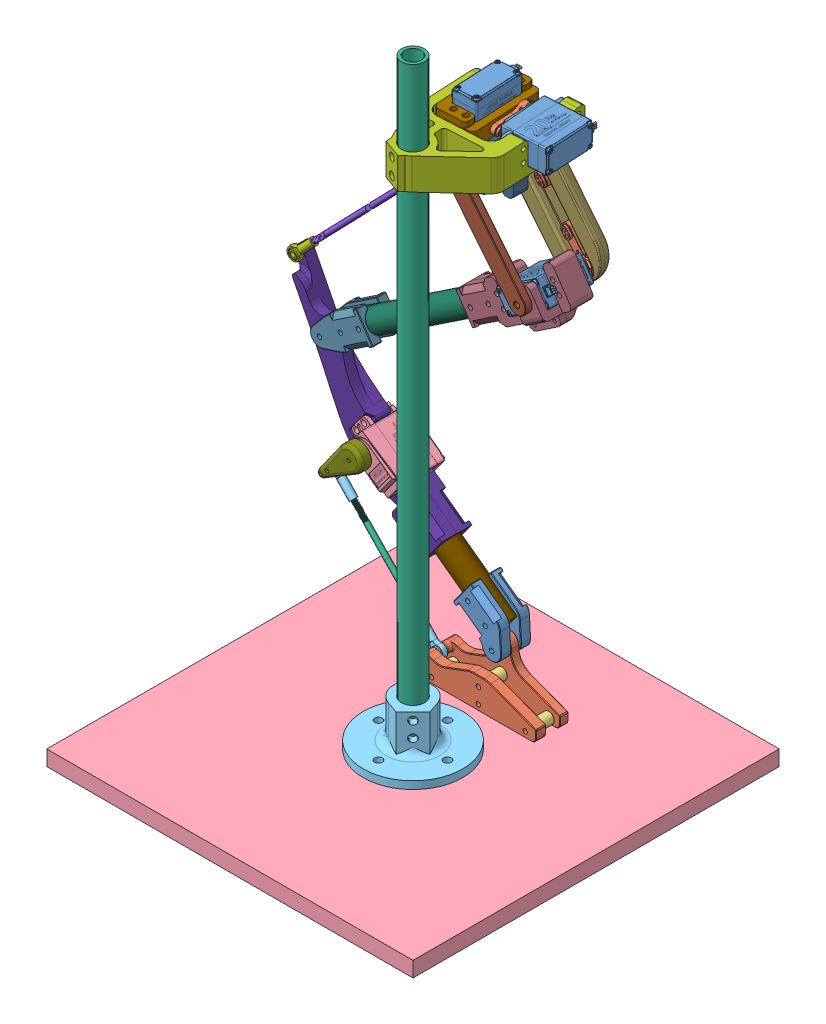
SolidWorks assembly Assembly 1 - updated tolerances, configuration Default. Lengths in mm.
Overall size (328.16 522.22 516.1).
41 component instances, 25 part files, 59 mates.
Components (placement in the parent):
- Servo_Body^Assembly 1 - updated tolerances-1: Servo_Body^Assembly 1 - updated tolerances [Default] at (148.642 192.4655 -24.1058) x (-0.998744 0 0.050107) z (0.050107 0 0.998744) size (20.1 45.99 55.6) (virtual)
- Servo_Arm^Assembly 1 - updated tolerances-2: Servo_Arm^Assembly 1 - updated tolerances [Default] at (148.642 192.4655 -24.1058) x (0 0 1) z (1 0 0) size (14.5 6.95 35.53) (virtual)
- Servo_Arm^Assembly 1 - updated tolerances-4: Servo_Arm^Assembly 1 - updated tolerances [Default] at (147.142 155.4655 -30.1058) x (0.778746 0.62734 0) z (-0.62734 0.778746 0) size (14.5 6.95 35.53) (virtual)
- Servo_Body^Assembly 1 - updated tolerances-3: Servo_Body^Assembly 1 - updated tolerances [Default] at (147.142 155.4655 -30.1058) x (0 1 0) z (-1 0 0) size (20.1 45.99 55.6) (virtual)
- Servo Arm^Assembly 1 - updated tolerances-1: Servo Arm^Assembly 1 - updated tolerances [Default] at (54.4738 -91.7116 -17.6058) x (-0.678962 0.734173 0) z (0.734173 0.678962 0) size (14.5 6.95 35.53) (virtual)
- Servo Body^Assembly 1 - updated tolerances-1: Servo Body^Assembly 1 - updated tolerances [Default] at (54.4738 -91.7116 -17.6058) x (0.591048 0.806636 0) z (0.806636 -0.591048 0) size (20.1 45.99 55.6) (virtual)
- Servo_Body^Assembly 1 - updated tolerances-4: Servo_Body^Assembly 1 - updated tolerances [Default] at (197.3292 93.1658 -30.1058) x (-0.556075 0.831132 0) z (-0.831132 -0.556075 0) size (20.1 45.99 55.6) (virtual)
- Servo_Arm^Assembly 1 - updated tolerances-5: Servo_Arm^Assembly 1 - updated tolerances [Default] at (185.4452 198.4655 -28.956) x (0 -1 0) z (-0.050107 0 -0.998744) size (14.5 6.95 35.53) (virtual)
- Servo_Body^Assembly 1 - updated tolerances-5: Servo_Body^Assembly 1 - updated tolerances [Default] at (184.4465 198.4655 -28.9059) x (0 1 0) z (0.050107 0 0.998744) size (20.1 45.99 55.6) (virtual)
- Servo_Arm^Assembly 1 - updated tolerances-6: Servo_Arm^Assembly 1 - updated tolerances [Default] at (197.3292 93.1658 -30.1058) x (-0.778746 -0.62734 0) z (0.62734 -0.778746 0) size (14.5 6.95 35.53) (virtual)
- M4 Linkage 2^Assembly 1 - updated tolerances-2: M4 Linkage 2^Assembly 1 - updated tolerances [Default] at (57.0233 -140.42 -5.5558) x (-0.707835 -0.683211 -0.17942) z (0.694481 -0.719511 0) size (18.79 7.88 136) (virtual)
  - M3 Ball Joint Rod End^M4 Linkage 2_Assembly 1 - updated tolerances-1: M3 Ball Joint Rod End^M4 Linkage 2_Assembly 1 - updated tolerances [59935K14] at (0 0 75) x (-0.983773 0.17942 0) z (0.17942 0.983773 0) size (11 28.3 6) (virtual)
  - M4 Connecting Rod^M4 Linkage 2_Assembly 1 - updated tolerances-1: M4 Connecting Rod^M4 Linkage 2_Assembly 1 - updated tolerances [6516K132] at origin size (4.62 4.16 100.16) (virtual)
  - M3 Ball Joint Rod End^M4 Linkage 2_Assembly 1 - updated tolerances-2: M3 Ball Joint Rod End^M4 Linkage 2_Assembly 1 - updated tolerances [59935K14] at (0 0 -25) x (0.983773 -0.17942 0) z (0.17942 0.983773 0) size (11 28.3 6) (virtual)
- M4 Linkage 1^Assembly 1 - updated tolerances-3: M4 Linkage 1^Assembly 1 - updated tolerances [Default] at (45.9964 73.679 -18.6558) x (-0.70731 0.683755 -0.17942) z (-0.695033 -0.718977 0) size (11.9 7.88 190) (virtual)
  - M3 Ball Joint Rod End^M4 Linkage 1_Assembly 1 - updated tolerances-1: M3 Ball Joint Rod End^M4 Linkage 1_Assembly 1 - updated tolerances [59935K14] at (0 0 75) x (-0.983773 0.17942 0) z (0.17942 0.983773 0) size (11 28.3 6) (virtual)
  - M4 Connecting Rod^M4 Linkage 1_Assembly 1 - updated tolerances-1: M4 Connecting Rod^M4 Linkage 1_Assembly 1 - updated tolerances [6516K132] at origin size (4.62 4.16 154.16) (virtual)
  - M3 Ball Joint Rod End^M4 Linkage 1_Assembly 1 - updated tolerances-2: M3 Ball Joint Rod End^M4 Linkage 1_Assembly 1 - updated tolerances [59935K14] at (0 0 -79) x (0.983773 -0.17942 0) z (0.17942 0.983773 0) size (11 28.3 6) (virtual)
- Hip 1.STL^Assembly 1 - updated tolerances-3: Hip 1.STL^Assembly 1 - updated tolerances [Default] at (149.1431 198.4655 -14.1184) x (0.050107 0 0.998744) z (0.998744 0 -0.050107) size (60 16.5 32) (virtual)
- Hip 2^Assembly 1 - updated tolerances-3: Hip 2^Assembly 1 - updated tolerances [Default] at (137.142 155.4655 -24.1058) x (1 0 0) z (0 1 0) size (62.55 33.6 37) (virtual)
- Thigh inner^Assembly 1 - updated tolerances-1: Thigh inner^Assembly 1 - updated tolerances [Default] at (147.142 155.4655 6.4942) x (0.62734 -0.778746 0) z (0.778746 0.62734 0) size (95 6 15) (virtual)
- Thigh Outer^Assembly 1 - updated tolerances-1: Thigh Outer^Assembly 1 - updated tolerances [Default] at (147.142 155.4655 -54.1058) x (0.62734 -0.778746 0) z (-0.778746 -0.62734 0) size (101 12.91 45) (virtual)
- Foreleg^Assembly 1 - updated tolerances-1: Foreleg^Assembly 1 - updated tolerances [Default] at (20.1296 -30.1009 -17.6058) x (0.98242 -0.186684 0) z (0 0 1) size (196.97 194.09 159.12) (virtual)
  - Foreleg upper^Foreleg_Assembly 1 - updated tolerances-2: Foreleg upper^Foreleg_Assembly 1 - updated tolerances [Default] at (143.9453 147.1654 -6.5) x (-0.71271 -0.701458 0) z (0.701458 -0.71271 0) size (90 34.23 40) (virtual)
  - Foreleg lower^Foreleg_Assembly 1 - updated tolerances-1: Foreleg lower^Foreleg_Assembly 1 - updated tolerances [Default<As Machined>] at (211.6528 213.804 0) x (-0.593335 -0.804955 0) z (0 0 1) size (54.23 29.24 25) (virtual)
  - Pipe^Foreleg_Assembly 1 - updated tolerances-1: Pipe^Foreleg_Assembly 1 - updated tolerances [Default] at (-15.6593 20.1147 -3.3296) x (0.23303 0.779273 0.581748) z (-0.581748 0.59108 -0.558742) size (127.4 125.81 19.05) (virtual)
- Servo Cover^Assembly 1 - updated tolerances-1: Servo Cover^Assembly 1 - updated tolerances [Default] at (-100.0173 35.5664 -15.2721) x (0.997673 -0.009925 0.067458) z (-0.065704 0.124465 0.990046) size (37 36.07 11.56) (virtual)
- Shin^Assembly 1 - updated tolerances-1: Shin^Assembly 1 - updated tolerances [Default] at (-9.6004 -3.0399 -16.3225) x (0.995998 0.08937 0) z (0 0 1) size (171.31 218.62 25) (virtual)
  - Shin^Shin_Assembly 1 - updated tolerances-1: Shin^Shin_Assembly 1 - updated tolerances [Default] at (26.0363 -25.7805 -1.2832) size (126.76 169.15 25) (virtual)
  - shin pipe^Shin_Assembly 1 - updated tolerances-1: shin pipe^Shin_Assembly 1 - updated tolerances [Default] at (155.3385 -180.9229 -1.2832) x (0.232016 0.263552 0.936327) z (-0.618699 -0.702794 0.351128) size (19.05 90 19.05) (virtual)
  - Ankle^Shin_Assembly 1 - updated tolerances-1: Ankle^Shin_Assembly 1 - updated tolerances [Default] at (-51.7153 42.6675 -1.2832) size (38.53 48.45 25) (virtual)
- Foot^Assembly 1 - updated tolerances-1: Foot^Assembly 1 - updated tolerances [Default] at (-44.7227 54.2416 -17.6058) size (97 45.1 27) (virtual)
  - foot^Foot_Assembly 1 - updated tolerances-1: foot^Foot_Assembly 1 - updated tolerances [Default] at (206.6131 -235.2675 0) size (97 45.1 27) (virtual)
  - Foot Spacer^Foot_Assembly 1 - updated tolerances-1: Foot Spacer^Foot_Assembly 1 - updated tolerances [Default] at (206.6131 -255.7675 3.5) size (9.2 9.2 11.5) (virtual)
  - Foot Spacer^Foot_Assembly 1 - updated tolerances-2: Foot Spacer^Foot_Assembly 1 - updated tolerances [Default] at (245.6131 -268.2675 3.5) size (9.2 9.2 11.5) (virtual)
  - Foot Spacer^Foot_Assembly 1 - updated tolerances-3: Foot Spacer^Foot_Assembly 1 - updated tolerances [Default] at (167.6131 -268.2675 3.5) size (9.2 9.2 11.5) (virtual)
  - Foot Spacer^Foot_Assembly 1 - updated tolerances-4: Foot Spacer^Foot_Assembly 1 - updated tolerances [Default] at (206.6131 -268.2675 3.5) size (9.2 9.2 11.5) (virtual)
- Wooden Base^Assembly 1 - updated tolerances-1: Wooden Base^Assembly 1 - updated tolerances [Default] at origin size (304.8 12.7 304.8) (virtual)
- Adaptor^Assembly 1 - updated tolerances-1: Adaptor^Assembly 1 - updated tolerances [Default] at origin size (82.85 38.1 82.85) (virtual)
- Test Pipe^Assembly 1 - updated tolerances-1: Test Pipe^Assembly 1 - updated tolerances [Default] at (131.6422 -241.4727 56.997) x (-0.103745 0.71271 0.693744) z (-0.989002 0 -0.147899) size (369.72 364.31 19.05) (virtual)
- Test Bench Adaptor v1^Assembly 1 - updated tolerances-1: Test Bench Adaptor v1^Assembly 1 - updated tolerances [Default] at (190.94 198.4655 -19.2191) x (0.050107 0 0.998744) z (0 -1 0) size (113.76 72 26) (virtual)
Mates (geometry in assembly coordinates):
- Coincident1: coincident anti-aligned: plane of Servo Body^Assembly 1-1 through (54.4738 -91.7116 0.7942) normal (0 0 1); plane of Servo Arm^Assembly 1-1 through (54.4738 -91.7116 0.7942) normal (0 0 -1)
- Concentric1: concentric anti-aligned: cylinder of Servo Arm^Assembly 1-1 through (54.4738 -91.7116 0.7942) axis (0 0 -1) radius 2.5; cylinder of Servo Body^Assembly 1-1 through (54.4738 -91.7116 -4.1058) axis (0 0 1) radius 3.8
- Concentric15: concentric aligned: cylinder of Servo Body^Assembly 1-1 through (84.8547 -107.774 -23.9698) axis (0 0 1) radius 2.25; cylinder of Shin^Assembly 1-1/Shin^Shin_Assembly 1-1 through (84.8547 -107.774 -30.1058) axis (0 0 1) radius 1.9
- Concentric16: concentric aligned: cylinder of Servo Body^Assembly 1-1 through (78.9442 -115.8404 -23.9698) axis (0 0 1) radius 2.25; cylinder of Shin^Assembly 1-1/Shin^Shin_Assembly 1-1 through (78.9442 -115.8404 -30.1058) axis (0 0 1) radius 1.9
- Coincident10: coincident anti-aligned: plane of Servo Body^Assembly 1-1 through (81.5725 -100.4102 -17.6058) normal (0 0 -1); plane of Shin^Assembly 1-1/Shin^Shin_Assembly 1-1 through (93.3552 -103.4651 -17.6058) normal (0 0 1)
- Width5: width anti-aligned: plane of Foot^Assembly 1 - updated tolerances-1/foot^Foot_Assembly 1 - updated tolerances-1 through (117.7904 -203.3773 -14.1058) normal (0 0 1); plane of Shin^Assembly 1 - updated tolerances-1/Ankle^Shin_Assembly 1 - updated tolerances-1 through (117.7904 -203.3773 -21.1058) normal (0 0 -1); plane of Foot^Assembly 1 - updated tolerances-1/foot^Foot_Assembly 1 - updated tolerances-1 through (161.9449 -200.8322 -13.6058) normal (0 0 -1); plane of Shin^Assembly 1 - updated tolerances-1/Ankle^Shin_Assembly 1 - updated tolerances-1 through (161.9449 -200.8322 -21.6058) normal (0 0 1)
- Concentric5: concentric anti-aligned: cylinder of Servo_Arm^Assembly 1-2 through (148.642 174.0655 -24.1058) axis (0 1 0) radius 2.5; cylinder of Servo_Body^Assembly 1-1 through (148.642 178.9655 -24.1058) axis (0 -1 0) radius 3.8
- Coincident5: coincident anti-aligned: plane of Servo_Body^Assembly 1-1 through (148.642 174.0655 -24.1058) normal (0 -1 0); plane of Servo_Arm^Assembly 1-2 through (148.642 174.0655 -24.1058) normal (0 1 0)
- Concentric20: concentric anti-aligned: circle of Servo_Arm^Assembly 1-2; cylinder of Hip 2^Assembly 1-3 through (124.142 139.4655 -24.1058) axis (0 1 0) radius 1.4
- Concentric21: concentric anti-aligned: circle of Servo_Arm^Assembly 1-2; cylinder of Hip 2^Assembly 1-3 through (148.642 139.4655 -24.1058) axis (0 1 0) radius 1.4
- Coincident11: coincident anti-aligned: plane of Servo_Arm^Assembly 1-2 through (138.292 171.4655 -10.3058) normal (0 -1 0); plane of Hip 2^Assembly 1-3 through (137.142 171.4655 -30.1058) normal (0 1 0)
- Concentric22: concentric anti-aligned: cylinder of Servo_Body^Assembly 1-2 through (197.3292 93.1658 -43.6058) axis (0 0 -1) radius 3.8; cylinder of Servo_Arm^Assembly 1-3 through (197.3292 93.1658 -48.5058) axis (0 0 1) radius 2.5
- Coincident12: coincident anti-aligned: plane of Servo_Body^Assembly 1-2 through (197.3292 93.1658 -48.5058) normal (0 0 -1); plane of Servo_Arm^Assembly 1-3 through (197.3292 93.1658 -48.5058) normal (0 0 1)
- Concentric35: concentric anti-aligned: cylinder of Servo_Arm^Assembly 1-4 through (147.142 155.4655 -48.5058) axis (0 0 1) radius 2.5; cylinder of Servo_Body^Assembly 1-3 through (147.142 155.4655 -43.6058) axis (0 0 -1) radius 3.8
- Coincident25: coincident anti-aligned: plane of Servo_Arm^Assembly 1-4 through (147.142 155.4655 -48.5058) normal (0 0 1); plane of Servo_Body^Assembly 1-3 through (147.142 155.4655 -48.5058) normal (0 0 -1)
- Concentric36: concentric aligned: circle of Servo_Body^Assembly 1-3; cylinder of Hip 2^Assembly 1-3 through (113.142 160.4655 -18.1058) axis (0 0 -1) radius 1.9
- Concentric37: concentric aligned: circle of Servo_Body^Assembly 1-3; cylinder of Hip 2^Assembly 1-3 through (161.142 160.4655 -18.1058) axis (0 0 -1) radius 1.9
- Coincident26: coincident anti-aligned: plane of Servo_Body^Assembly 1-3 through (120.142 164.4655 -30.1058) normal (0 0 1); plane of Hip 2^Assembly 1-3 through (137.142 155.4655 -30.1058) normal (0 0 -1)
- Coincident27: coincident anti-aligned: plane of Servo_Body^Assembly 1-2 through (169.8839 85.632 -30.1058) normal (0 0 1); plane of Foreleg^Assembly 1 - updated tolerances-1/Foreleg upper^Foreleg_Assembly 1 - updated tolerances-2 through (189.0179 87.605 -30.1058) normal (0 0 -1)
- Concentric50: concentric anti-aligned: cylinder of Shin^Assembly 1-1/Shin^Shin_Assembly 1-1 through (18.6358 -26.3903 -5.1058) axis (0 0 -1) radius 2.1; cylinder of Foreleg^Assembly 1 - updated tolerances-1/Foreleg lower^Foreleg_Assembly 1 - updated tolerances-1 through (18.6358 -26.3903 -30.1058) axis (0 0 1) radius 1.9
- Width7: width anti-aligned: plane of Foreleg^Assembly 1 - updated tolerances-1/Foreleg lower^Foreleg_Assembly 1 - updated tolerances-1 through (18.6358 -26.3903 -5.1058) normal (0 0 1); plane of Foreleg^Assembly 1 - updated tolerances-1/Foreleg lower^Foreleg_Assembly 1 - updated tolerances-1 through (18.6358 -26.3903 -30.1058) normal (0 0 -1); plane of Shin^Assembly 1 - updated tolerances-1/Shin^Shin_Assembly 1 - updated tolerances-1 through (18.6358 -26.3903 -21.6058) normal (0 0 -1); plane of Shin^Assembly 1 - updated tolerances-1/Shin^Shin_Assembly 1 - updated tolerances-1 through (18.6358 -26.3903 -13.6058) normal (0 0 1)
- Concentric53: concentric anti-aligned: cylinder of Servo_Body^Assembly 1-2 through (206.1846 105.1065 -23.7418) axis (0 0 -1) radius 2.25; cylinder of Foreleg^Assembly 1 - updated tolerances-1/Foreleg upper^Foreleg_Assembly 1 - updated tolerances-2 through (206.1846 105.1065 -30.1058) axis (0 0 1) radius 1.9
- Concentric54: concentric anti-aligned: cylinder of Servo_Body^Assembly 1-2 through (211.7454 96.7952 -23.7418) axis (0 0 -1) radius 2.25; cylinder of Foreleg^Assembly 1 - updated tolerances-1/Foreleg upper^Foreleg_Assembly 1 - updated tolerances-2 through (211.7454 96.7952 -30.1058) axis (0 0 1) radius 1.9
- Delete later: parallel: line of Hip 2^Assembly 1-3 through (157.192 167.4655 3.4942) axis (-1 0 0)
- Origin mate: coordinate: point of Foot^Assembly 1-1
- Concentric76: concentric anti-aligned: cylinder of M4 Linkage 2^Assembly 1-2/M3 Ball Joint Rod End^M4 Linkage 2_Assembly 1-2 through (30.9803 -113.4384 -2.5558) axis (0 0 -1) radius 2; cylinder of Servo Cover^Assembly 1-1 through (30.9803 -113.4384 -2.6058) axis (0 0 1) radius 1.4
- Concentric77: concentric aligned: cylinder of Servo Arm^Assembly 1-1 through (54.4738 -91.7116 -2.6058) axis (0 0 1) radius 7.25; cylinder of Servo Cover^Assembly 1-1 through (54.4738 -91.7116 -2.6058) axis (0 0 1) radius 7.55
- Concentric78: concentric aligned: circle of Servo Arm^Assembly 1-1; cylinder of Servo Cover^Assembly 1-1 through (36.4866 -108.3462 -2.6058) axis (0 0 1) radius 4.1
- Coincident43: coincident anti-aligned: plane of Servo Arm^Assembly 1-1 through (37.5055 -88.6073 3.3942) normal (0 0 1); plane of Servo Cover^Assembly 1-1 through (36.4866 -108.3462 3.3942) normal (0 0 -1)
- Concentric82: concentric aligned: cylinder of M4 Linkage 2^Assembly 1-2/M3 Ball Joint Rod End^M4 Linkage 2_Assembly 1-1 through (117.7904 -203.3773 -2.5558) axis (0 0 -1) radius 2; cylinder of Foot^Assembly 1 - updated tolerances-1/foot^Foot_Assembly 1 - updated tolerances-1 through (117.7904 -203.3773 5.8942) axis (0 0 -1) radius 1.4
- Concentric83: concentric aligned: cylinder of M4 Linkage 1^Assembly 1-3/M3 Ball Joint Rod End^M4 Linkage 1_Assembly 1-2 through (109.592 139.4655 -15.6558) axis (0 0 -1) radius 2; cylinder of Hip 2^Assembly 1-3 through (109.592 139.4655 3.4942) axis (0 0 -1) radius 1.4
- Concentric84: concentric aligned: cylinder of M4 Linkage 1^Assembly 1-3/M3 Ball Joint Rod End^M4 Linkage 1_Assembly 1-1 through (-14.819 10.7685 -15.6558) axis (0 0 -1) radius 2; cylinder of Shin^Assembly 1-1/Shin^Shin_Assembly 1-1 through (-14.819 10.7685 -5.1058) axis (0 0 -1) radius 1.4
- Distance1: distance = 0.5 mm anti-aligned: plane of M4 Linkage 2^Assembly 1-2/M3 Ball Joint Rod End^M4 Linkage 2_Assembly 1-2 through (31.118 -105.6614 -3.1058) normal (0 0 1); plane of Servo Cover^Assembly 1-1 through (30.9803 -113.4384 -2.6058) normal (0 0 -1)
- Concentric86: concentric aligned: cylinder of Thigh inner^Assembly 1-1 through (197.3292 93.1658 3.4942) axis (0 0 1) radius 2.1; cylinder of Foreleg^Assembly 1 - updated tolerances-1/Foreleg upper^Foreleg_Assembly 1 - updated tolerances-2 through (197.3292 93.1658 -6.5058) axis (0 0 1) radius 1.9
- Concentric2: concentric aligned: cylinder of Thigh inner^Assembly 1-1 through (147.142 155.4655 3.4942) axis (0 0 1) radius 2.1; cylinder of Hip 2^Assembly 1-3 through (147.142 155.4655 -6.5058) axis (0 0 1) radius 1.9
- Concentric87: concentric aligned: circle of Servo_Arm^Assembly 1-3; cylinder of Thigh Outer^Assembly 1-1 through (181.9594 112.2451 -51.1058) axis (0 0 -1) radius 1.4
- Coincident44: coincident anti-aligned: plane of Servo_Arm^Assembly 1-3 through (180.0895 92.5685 -51.1058) normal (0 0 -1); plane of Thigh Outer^Assembly 1-1 through (147.142 155.4655 -51.1058) normal (0 0 1)
- Coincident45: coincident anti-aligned: plane of Servo_Arm^Assembly 1-4 through (164.3817 156.0627 -51.1058) normal (0 0 -1); plane of Thigh Outer^Assembly 1-1 through (147.142 155.4655 -51.1058) normal (0 0 1)
- Concentric88: concentric aligned: circle of Servo_Arm^Assembly 1-4; cylinder of Thigh Outer^Assembly 1-1 through (162.5118 136.3862 -51.1058) axis (0 0 -1) radius 1.4
- Concentric89: concentric aligned: cylinder of Servo_Arm^Assembly 1-3 through (197.3292 93.1658 -50.1058) axis (0 0 -1) radius 3.85; cylinder of Thigh Outer^Assembly 1-1 through (197.3292 93.1658 -45.1058) axis (0 0 -1) radius 1.4
- Concentric90: concentric aligned: cylinder of Servo_Arm^Assembly 1-4 through (147.142 155.4655 -45.1058) axis (0 0 -1) radius 7.25; cylinder of Thigh Outer^Assembly 1-1 through (147.142 155.4655 -45.1058) axis (0 0 -1) radius 1.4
- Coincident46: coincident anti-aligned: plane of Foreleg^Assembly 1 - updated tolerances-1/Foreleg upper^Foreleg_Assembly 1 - updated tolerances-2 through (233.1416 117.1264 3.4942) normal (0 0 1); plane of Thigh inner^Assembly 1-1 through (147.142 155.4655 3.4942) normal (0 0 -1)
- Concentric91: concentric aligned: cylinder of Servo_Body^Assembly 1-1 through (142.9468 198.8294 -37.8377) axis (0 -1 0) radius 2.25; cylinder of Copy of Hip 1 B.STL^Assembly 1 - updated tolerances-3 through (142.9468 204.4655 -37.8377) axis (0 -1 0) radius 2.4
- Concentric92: concentric aligned: cylinder of Servo_Body^Assembly 1-1 through (152.9342 198.8294 -38.3387) axis (0 -1 0) radius 2.25; cylinder of Copy of Hip 1 B.STL^Assembly 1 - updated tolerances-3 through (152.9342 204.4655 -38.3387) axis (0 -1 0) radius 2.4
- Coincident47: coincident anti-aligned: plane of Servo_Body^Assembly 1-1 through (141.0062 192.4655 3.3113) normal (0 1 0); plane of Copy of Hip 1 B.STL^Assembly 1 - updated tolerances-3 through (149.1431 192.4655 -14.1184) normal (0 -1 0)
- Concentric93: concentric anti-aligned: circle of Servo_Arm^Assembly 1-5; circle of Hip 1^Assembly 1-1
- Concentric94: concentric aligned: cylinder of Servo_Arm^Assembly 1-5 through (167.0683 198.4655 -28.034) axis (0.998744 0 -0.050107) radius 2.5; cylinder of Copy of Hip 1 B.STL^Assembly 1 - updated tolerances-3 through (132.5118 198.4655 -26.3003) axis (0.998744 0 -0.050107) radius 1.45
- Concentric95: concentric anti-aligned: cylinder of Servo_Arm^Assembly 1-5 through (167.0683 198.4655 -28.034) axis (0.998744 0 -0.050107) radius 2.5; cylinder of Servo_Body^Assembly 1-4 through (170.0645 198.4655 -28.1843) axis (-0.998744 0 0.050107) radius 1.25
- Coincident48: coincident anti-aligned: plane of Servo_Arm^Assembly 1-5 through (170.9826 184.6655 -17.8674) normal (0.998744 0 -0.050107); plane of Servo_Body^Assembly 1-4 through (170.464 198.4655 -28.2044) normal (-0.998744 0 0.050107)
- Coincident49: coincident anti-aligned: plane of Servo_Arm^Assembly 1-5 through (164.9902 184.6655 -17.5667) normal (-0.998744 0 0.050107); plane of Copy of Hip 1 B.STL^Assembly 1 - updated tolerances-3 through (165.123 192.4655 -14.9201) normal (0.998744 0 -0.050107)
- Concentric96: concentric aligned: cylinder of Adaptor^Assembly 1-1 through (152.4 -190.5 50.8) axis (0 -1 0) radius 9.675; cylinder of Test Pipe^Assembly 1-1 through (152.4 271.4 50.8) axis (0 -1 0) radius 9.525
- Coincident50: coincident aligned: plane of Wooden Base^Assembly 1-1 through (0 -228.6 0) normal (0 1 0); circle of Test Pipe^Assembly 1-1
- Distance2: distance = 0.5 mm anti-aligned: plane of M4 Linkage 1^Assembly 1-3/M3 Ball Joint Rod End^M4 Linkage 1_Assembly 1-2 through (117.3691 139.5971 -21.1058) normal (0 0 -1); plane of Hip 2^Assembly 1-3 through (137.142 155.4655 -21.6058) normal (0 0 1)
- Concentric97: concentric anti-aligned: circle of Servo_Body^Assembly 1-4; cylinder of Test Bench Adaptor v1^Assembly 1-1 through (198.135 203.4655 4.4501) axis (-0.998744 0 0.050107) radius 1.9
- Concentric98: concentric aligned: cylinder of Servo_Body^Assembly 1-4 through (192.5061 193.4655 4.7326) axis (-0.998744 0 0.050107) radius 2.25; cylinder of Test Bench Adaptor v1^Assembly 1-1 through (198.135 193.4655 4.4501) axis (-0.998744 0 0.050107) radius 1.9
- Coincident53: coincident anti-aligned: plane of Servo_Body^Assembly 1-4 through (185.7993 207.4655 -1.9398) normal (0.998744 0 -0.050107); plane of Test Bench Adaptor v1^Assembly 1-1 through (186.8627 299.5109 19.2552) normal (-0.998744 0 0.050107)
- Concentric99: concentric aligned: cylinder of Test Pipe^Assembly 1-1 through (152.4 271.4 50.8) axis (0 -1 0) radius 9.525; cylinder of Test Bench Adaptor v1^Assembly 1-1 through (152.4 299.5109 50.8) axis (0 -1 0) radius 9.725
- Concentric100: concentric aligned: cylinder of Shin^Assembly 1-1/Ankle^Shin_Assembly 1-1 through (161.8904 -181.0259 -5.1058) axis (0 0 -1) radius 1.9; cylinder of Foot^Assembly 1 - updated tolerances-1/foot^Foot_Assembly 1 - updated tolerances-1 through (161.8904 -181.0259 -14.1058) axis (0 0 -1) radius 2.1
- Parallel3: parallel: line of Foot^Assembly 1 - updated tolerances-1/foot^Foot_Assembly 1 - updated tolerances-1 through (205.8904 -218.5259 -21.1058) axis (-1 0 0); plane of Wooden Base^Assembly 1-1 through (0 -228.6 0) normal (0 1 0)
